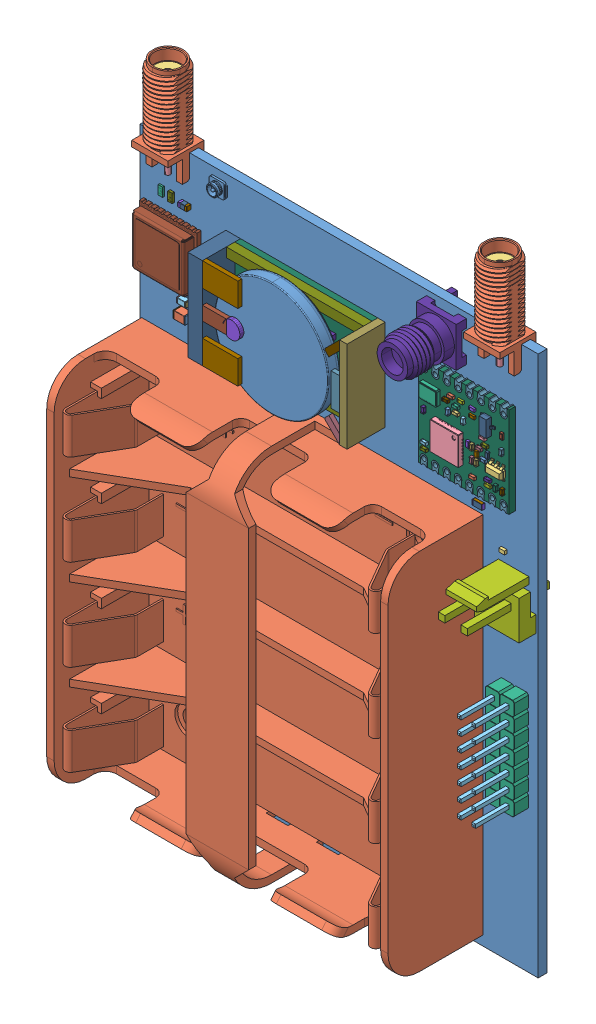
SolidWorks assembly Печатная плата Peggy Tracker, configuration Default. Lengths in mm. (continued)
Components (placement in the parent): (continued)
- Печатная плата Peggy Tracker(2)^Печатная плата Peggy Tracker-1: Печатная плата Peggy Tracker(2)^Печатная плата Peggy Tracker [Default] at origin size (70 108.1 20.64) (virtual) (continued)
  - DD2^Печатная плата Peggy Tracker(2)_Печатная плата Peggy Tracker-1: DD2^Печатная плата Peggy Tracker(2)_Печатная плата Peggy Tracker [Default] at origin size (15.9 16 2.23) (virtual) (continued)
    - User_Library-RFM96W^DD2_Печатная плата Peggy Tracker(2)_Печатная плата Peggy Tracker-1: User_Library-RFM96W^DD2_Печатная плата Peggy Tracker(2)_Печатная плата Peggy Tracker [Default] at (50.075 85.102 1.15) x (0 -1 0) z (0 0 1) size (16 15.9 2.23) (virtual) (continued)
      - Designator31^User_Library-RFM96W_DD2_Печатная плата Peggy Tracker(2)_Печатная плата Peggy Tracker-1: Designator31^User_Library-RFM96W_DD2_Печатная плата Peggy Tracker(2)_Печатная плата Peggy Tracker [Default] at origin size (1 0.5 0.5) (virtual) (continued)
        - Cap0402^Designator31_User_Library-RFM96W_DD2_Печатная плата Peggy Tracker(2)_Печатная плата Peggy Tracker-1: Cap0402^Designator31_User_Library-RFM96W_DD2_Печатная плата Peggy Tracker(2)_Печатная плата Peggy Tracker [По умолчанию] at (8.636 9.652 0) x (-1 0 0) z (0 1 0) size (1 0.5 0.5) (virtual)
      - Designator32^User_Library-RFM96W_DD2_Печатная плата Peggy Tracker(2)_Печатная плата Peggy Tracker-1: Designator32^User_Library-RFM96W_DD2_Печатная плата Peggy Tracker(2)_Печатная плата Peggy Tracker [Default] at origin size (1 0.5 0.5) (virtual)
        - Cap0402^Designator32_User_Library-RFM96W_DD2_Печатная плата Peggy Tracker(2)_Печатная плата Peggy Tracker-1: Cap0402^Designator32_User_Library-RFM96W_DD2_Печатная плата Peggy Tracker(2)_Печатная плата Peggy Tracker [По умолчанию] at (10.668 9.652 0) x (-1 0 0) z (0 1 0) size (1 0.5 0.5) (virtual)
      - Free-Models^User_Library-RFM96W_DD2_Печатная плата Peggy Tracker(2)_Печатная плата Peggy Tracker-1: Free-Models^User_Library-RFM96W_DD2_Печатная плата Peggy Tracker(2)_Печатная плата Peggy Tracker [Default] at origin size (16 15.3 1.16) (virtual)
        - Goldcontact^Free-Models_User_Library-RFM96W_DD2_Печатная плата Peggy Tracker(2)_Печатная плата Peggy Tracker-1: Goldcontact^Free-Models_User_Library-RFM96W_DD2_Печатная плата Peggy Tracker(2)_Печатная плата Peggy Tracker [По умолчанию] at (0.56 1 -1.14) x (-1 0 0) z (0 1 0) size (1.77 1.16 1.3) (virtual)
        - Goldcontact^Free-Models_User_Library-RFM96W_DD2_Печатная плата Peggy Tracker(2)_Печатная плата Peggy Tracker-2: Goldcontact^Free-Models_User_Library-RFM96W_DD2_Печатная плата Peggy Tracker(2)_Печатная плата Peggy Tracker [По умолчанию] at (0.56 3 -1.14) x (-1 0 0) z (0 1 0) size (1.77 1.16 1.3) (virtual)
        - Goldcontact^Free-Models_User_Library-RFM96W_DD2_Печатная плата Peggy Tracker(2)_Печатная плата Peggy Tracker-3: Goldcontact^Free-Models_User_Library-RFM96W_DD2_Печатная плата Peggy Tracker(2)_Печатная плата Peggy Tracker [По умолчанию] at (0.56 5 -1.14) x (-1 0 0) z (0 1 0) size (1.77 1.16 1.3) (virtual)
        - Goldcontact^Free-Models_User_Library-RFM96W_DD2_Печатная плата Peggy Tracker(2)_Печатная плата Peggy Tracker-4: Goldcontact^Free-Models_User_Library-RFM96W_DD2_Печатная плата Peggy Tracker(2)_Печатная плата Peggy Tracker [По умолчанию] at (0.56 7 -1.14) x (-1 0 0) z (0 1 0) size (1.77 1.16 1.3) (virtual)
        - Goldcontact^Free-Models_User_Library-RFM96W_DD2_Печатная плата Peggy Tracker(2)_Печатная плата Peggy Tracker-5: Goldcontact^Free-Models_User_Library-RFM96W_DD2_Печатная плата Peggy Tracker(2)_Печатная плата Peggy Tracker [По умолчанию] at (0.56 9 -1.14) x (-1 0 0) z (0 1 0) size (1.77 1.16 1.3) (virtual)
        - Goldcontact^Free-Models_User_Library-RFM96W_DD2_Печатная плата Peggy Tracker(2)_Печатная плата Peggy Tracker-6: Goldcontact^Free-Models_User_Library-RFM96W_DD2_Печатная плата Peggy Tracker(2)_Печатная плата Peggy Tracker [По умолчанию] at (0.56 11 -1.14) x (-1 0 0) z (0 1 0) size (1.77 1.16 1.3) (virtual)
        - Goldcontact^Free-Models_User_Library-RFM96W_DD2_Печатная плата Peggy Tracker(2)_Печатная плата Peggy Tracker-7: Goldcontact^Free-Models_User_Library-RFM96W_DD2_Печатная плата Peggy Tracker(2)_Печатная плата Peggy Tracker [По умолчанию] at (0.56 13 -1.14) x (-1 0 0) z (0 1 0) size (1.77 1.16 1.3) (virtual)
        - Goldcontact^Free-Models_User_Library-RFM96W_DD2_Печатная плата Peggy Tracker(2)_Печатная плата Peggy Tracker-8: Goldcontact^Free-Models_User_Library-RFM96W_DD2_Печатная плата Peggy Tracker(2)_Печатная плата Peggy Tracker [По умолчанию] at (0.56 15 -1.14) x (-1 0 0) z (0 1 0) size (1.77 1.16 1.3) (virtual)
        - Goldcontact^Free-Models_User_Library-RFM96W_DD2_Печатная плата Peggy Tracker(2)_Печатная плата Peggy Tracker-9: Goldcontact^Free-Models_User_Library-RFM96W_DD2_Печатная плата Peggy Tracker(2)_Печатная плата Peggy Tracker [По умолчанию] at (15.442 15 -1.14) x (1 0 0) z (0 -1 0) size (1.77 1.16 1.3) (virtual)
        - Goldcontact^Free-Models_User_Library-RFM96W_DD2_Печатная плата Peggy Tracker(2)_Печатная плата Peggy Tracker-10: Goldcontact^Free-Models_User_Library-RFM96W_DD2_Печатная плата Peggy Tracker(2)_Печатная плата Peggy Tracker [По умолчанию] at (15.442 13 -1.14) x (1 0 0) z (0 -1 0) size (1.77 1.16 1.3) (virtual)
        - Goldcontact^Free-Models_User_Library-RFM96W_DD2_Печатная плата Peggy Tracker(2)_Печатная плата Peggy Tracker-11: Goldcontact^Free-Models_User_Library-RFM96W_DD2_Печатная плата Peggy Tracker(2)_Печатная плата Peggy Tracker [По умолчанию] at (15.442 11 -1.14) x (1 0 0) z (0 -1 0) size (1.77 1.16 1.3) (virtual)
        - Goldcontact^Free-Models_User_Library-RFM96W_DD2_Печатная плата Peggy Tracker(2)_Печатная плата Peggy Tracker-12: Goldcontact^Free-Models_User_Library-RFM96W_DD2_Печатная плата Peggy Tracker(2)_Печатная плата Peggy Tracker [По умолчанию] at (15.442 9 -1.14) x (1 0 0) z (0 -1 0) size (1.77 1.16 1.3) (virtual)
        - Goldcontact^Free-Models_User_Library-RFM96W_DD2_Печатная плата Peggy Tracker(2)_Печатная плата Peggy Tracker-13: Goldcontact^Free-Models_User_Library-RFM96W_DD2_Печатная плата Peggy Tracker(2)_Печатная плата Peggy Tracker [По умолчанию] at (15.442 7 -1.14) x (1 0 0) z (0 -1 0) size (1.77 1.16 1.3) (virtual)
        - Goldcontact^Free-Models_User_Library-RFM96W_DD2_Печатная плата Peggy Tracker(2)_Печатная плата Peggy Tracker-14: Goldcontact^Free-Models_User_Library-RFM96W_DD2_Печатная плата Peggy Tracker(2)_Печатная плата Peggy Tracker [По умолчанию] at (15.442 5 -1.14) x (1 0 0) z (0 -1 0) size (1.77 1.16 1.3) (virtual)
        - Goldcontact^Free-Models_User_Library-RFM96W_DD2_Печатная плата Peggy Tracker(2)_Печатная плата Peggy Tracker-15: Goldcontact^Free-Models_User_Library-RFM96W_DD2_Печатная плата Peggy Tracker(2)_Печатная плата Peggy Tracker [По умолчанию] at (15.442 3 -1.14) x (1 0 0) z (0 -1 0) size (1.77 1.16 1.3) (virtual)
        - Goldcontact^Free-Models_User_Library-RFM96W_DD2_Печатная плата Peggy Tracker(2)_Печатная плата Peggy Tracker-16: Goldcontact^Free-Models_User_Library-RFM96W_DD2_Печатная плата Peggy Tracker(2)_Печатная плата Peggy Tracker [По умолчанию] at (15.442 1 -1.14) x (1 0 0) z (0 -1 0) size (1.77 1.16 1.3) (virtual)
      - Board-15^User_Library-RFM96W_DD2_Печатная плата Peggy Tracker(2)_Печатная плата Peggy Tracker-1: Board-15^User_Library-RFM96W_DD2_Печатная плата Peggy Tracker(2)_Печатная плата Peggy Tracker [По умолчанию] at (0 0 -1.1204) size (15.9 15.9 1.12) (virtual)
  - D2^Печатная плата Peggy Tracker(2)_Печатная плата Peggy Tracker-1: D2^Печатная плата Peggy Tracker(2)_Печатная плата Peggy Tracker [Default] at origin size (4.9 6 1.75) (virtual)
    - User_Library-SOIC-8-1^D2_Печатная плата Peggy Tracker(2)_Печатная плата Peggy Tracker-1: User_Library-SOIC-8-1^D2_Печатная плата Peggy Tracker(2)_Печатная плата Peggy Tracker [По умолчанию] at (19.8999 49.3999 -1.5596) x (1 0 0) z (0 0 -1) size (4.9 6 1.75) (virtual)
  - D1^Печатная плата Peggy Tracker(2)_Печатная плата Peggy Tracker-1: D1^Печатная плата Peggy Tracker(2)_Печатная плата Peggy Tracker [Default] at origin size (6.6 6.6 1.2) (virtual)
    - TSSOP-20^D1_Печатная плата Peggy Tracker(2)_Печатная плата Peggy Tracker-1: TSSOP-20^D1_Печатная плата Peggy Tracker(2)_Печатная плата Peggy Tracker [По умолчанию] at (14.6001 18.2999 -1.5596) x (0 1 0) z (-1 0 0) size (6.6 1.2 6.6) (virtual)
  - C15^Печатная плата Peggy Tracker(2)_Печатная плата Peggy Tracker-1: C15^Печатная плата Peggy Tracker(2)_Печатная плата Peggy Tracker [Default] at origin size (1.6 3.2 1) (virtual)
    - SW3dPS-1206_SMD_Capacitor^C15_Печатная плата Peggy Tracker(2)_Печатная плата Peggy Tracker-1: SW3dPS-1206_SMD_Capacitor^C15_Печатная плата Peggy Tracker(2)_Печатная плата Peggy Tracker [По умолчанию] at (29.1 17.2 -1.5596) x (0 -1 0) z (1 0 0) size (3.2 1 1.6) (virtual)
  - C14^Печатная плата Peggy Tracker(2)_Печатная плата Peggy Tracker-1: C14^Печатная плата Peggy Tracker(2)_Печатная плата Peggy Tracker [Default] at origin size (3.2 1.6 1) (virtual)
    - SW3dPS-1206_SMD_Capacitor^C14_Печатная плата Peggy Tracker(2)_Печатная плата Peggy Tracker-1: SW3dPS-1206_SMD_Capacitor^C14_Печатная плата Peggy Tracker(2)_Печатная плата Peggy Tracker [По умолчанию] at (58.6 84.5 -1.5596) x (1 0 0) z (0 1 0) size (3.2 1 1.6) (virtual)
  - C13^Печатная плата Peggy Tracker(2)_Печатная плата Peggy Tracker-1: C13^Печатная плата Peggy Tracker(2)_Печатная плата Peggy Tracker [Default] at origin size (0.8 1.6 0.3) (virtual)
    - SW3dPS-0603_SMD_Capacitor^C13_Печатная плата Peggy Tracker(2)_Печатная плата Peggy Tracker-1: SW3dPS-0603_SMD_Capacitor^C13_Печатная плата Peggy Tracker(2)_Печатная плата Peggy Tracker [По умолчанию] at (15.5001 55.6001 -1.5596) x (0 1 0) z (-1 0 0) size (1.6 0.3 0.8) (virtual)
  - C12^Печатная плата Peggy Tracker(2)_Печатная плата Peggy Tracker-1: C12^Печатная плата Peggy Tracker(2)_Печатная плата Peggy Tracker [Default] at origin size (0.8 1.6 0.3) (virtual)
    - SW3dPS-0603_SMD_Capacitor^C12_Печатная плата Peggy Tracker(2)_Печатная плата Peggy Tracker-1: SW3dPS-0603_SMD_Capacitor^C12_Печатная плата Peggy Tracker(2)_Печатная плата Peggy Tracker [По умолчанию] at (21.6999 54.9999 -1.5596) x (0 -1 0) z (1 0 0) size (1.6 0.3 0.8) (virtual)
  - C11^Печатная плата Peggy Tracker(2)_Печатная плата Peggy Tracker-1: C11^Печатная плата Peggy Tracker(2)_Печатная плата Peggy Tracker [Default] at origin size (1.7 0.9 0.9) (virtual)
    - 5945466272^C11_Печатная плата Peggy Tracker(2)_Печатная плата Peggy Tracker-1: 5945466272^C11_Печатная плата Peggy Tracker(2)_Печатная плата Peggy Tracker [Default] at (17.1 44.6 -1.5596) x (1 0 0) z (0 0 -1) size (1.7 0.9 0.9) (virtual)
      - Terminal-3^5945466272_C11_Печатная плата Peggy Tracker(2)_Печатная плата Peggy Tracker-1: Terminal-3^5945466272_C11_Печатная плата Peggy Tracker(2)_Печатная плата Peggy Tracker [Default] at (-0.85 -0.45 0) size (1.7 0.9 0.9) (virtual)
        - Open_CASCADE_STEP_translator_6.8_5.1.1^Terminal-3_5945466272_C11_Печатная плата Peggy Tracker(2)_Печатная плата Peggy Tracker-1: Open_CASCADE_STEP_translator_6.8_5.1.1^Terminal-3_5945466272_C11_Печатная плата Peggy Tracker(2)_Печатная плата Peggy Tracker [По умолчанию] at origin size (0.2 0.9 0.9) (virtual)
        - Open_CASCADE_STEP_translator_6.8_5.1.2^Terminal-3_5945466272_C11_Печатная плата Peggy Tracker(2)_Печатная плата Peggy Tracker-1: Open_CASCADE_STEP_translator_6.8_5.1.2^Terminal-3_5945466272_C11_Печатная плата Peggy Tracker(2)_Печатная плата Peggy Tracker [По умолчанию] at origin size (0.2 0.9 0.9) (virtual)
      - Mid_Body-1^5945466272_C11_Печатная плата Peggy Tracker(2)_Печатная плата Peggy Tracker-1: Mid_Body-1^5945466272_C11_Печатная плата Peggy Tracker(2)_Печатная плата Peggy Tracker [Default] at (-0.85 -0.45 0) size (1.3 0.9 0.9) (virtual)
        - Open_CASCADE_STEP_translator_6.8_5.2.1^Mid_Body-1_5945466272_C11_Печатная плата Peggy Tracker(2)_Печатная плата Peggy Tracker-1: Open_CASCADE_STEP_translator_6.8_5.2.1^Mid_Body-1_5945466272_C11_Печатная плата Peggy Tracker(2)_Печатная плата Peggy Tracker [По умолчанию] at origin size (1.3 0.9 0.9) (virtual)
  - C10^Печатная плата Peggy Tracker(2)_Печатная плата Peggy Tracker-1: C10^Печатная плата Peggy Tracker(2)_Печатная плата Peggy Tracker [Default] at origin size (1.75 0.95 0.87) (virtual)
    - 5945472432^C10_Печатная плата Peggy Tracker(2)_Печатная плата Peggy Tracker-1: 5945472432^C10_Печатная плата Peggy Tracker(2)_Печатная плата Peggy Tracker [Default] at (20.5 34.6 -1.5596) x (-1 0 0) z (0 0 -1) size (1.75 0.95 0.87) (virtual)
      - Terminal-4^5945472432_C10_Печатная плата Peggy Tracker(2)_Печатная плата Peggy Tracker-1: Terminal-4^5945472432_C10_Печатная плата Peggy Tracker(2)_Печатная плата Peggy Tracker [Default] at (-0.875 -0.475 0) size (1.75 0.95 0.87) (virtual)
        - Open_CASCADE_STEP_translator_6.8_127.1.1^Terminal-4_5945472432_C10_Печатная плата Peggy Tracker(2)_Печатная плата Peggy Tracker-1: Open_CASCADE_STEP_translator_6.8_127.1.1^Terminal-4_5945472432_C10_Печатная плата Peggy Tracker(2)_Печатная плата Peggy Tracker [По умолчанию] at origin size (0.2 0.95 0.87) (virtual)
        - Open_CASCADE_STEP_translator_6.8_127.1.2^Terminal-4_5945472432_C10_Печатная плата Peggy Tracker(2)_Печатная плата Peggy Tracker-1: Open_CASCADE_STEP_translator_6.8_127.1.2^Terminal-4_5945472432_C10_Печатная плата Peggy Tracker(2)_Печатная плата Peggy Tracker [По умолчанию] at origin size (0.2 0.95 0.87) (virtual)
      - Mid_Body-2^5945472432_C10_Печатная плата Peggy Tracker(2)_Печатная плата Peggy Tracker-1: Mid_Body-2^5945472432_C10_Печатная плата Peggy Tracker(2)_Печатная плата Peggy Tracker [Default] at (-0.875 -0.475 0) size (1.35 0.95 0.87) (virtual)
        - Open_CASCADE_STEP_translator_6.8_127.2.1^Mid_Body-2_5945472432_C10_Печатная плата Peggy Tracker(2)_Печатная плата Peggy Tracker-1: Open_CASCADE_STEP_translator_6.8_127.2.1^Mid_Body-2_5945472432_C10_Печатная плата Peggy Tracker(2)_Печатная плата Peggy Tracker [По умолчанию] at origin size (1.35 0.95 0.87) (virtual)
  - C9^Печатная плата Peggy Tracker(2)_Печатная плата Peggy Tracker-1: C9^Печатная плата Peggy Tracker(2)_Печатная плата Peggy Tracker [Default] at origin size (1.75 0.95 0.87) (virtual)
    - 5945463072^C9_Печатная плата Peggy Tracker(2)_Печатная плата Peggy Tracker-1: 5945463072^C9_Печатная плата Peggy Tracker(2)_Печатная плата Peggy Tracker [Default] at (22 42.9 -1.5596) x (1 0 0) z (0 0 -1) size (1.75 0.95 0.87) (virtual)
      - Terminal-5^5945463072_C9_Печатная плата Peggy Tracker(2)_Печатная плата Peggy Tracker-1: Terminal-5^5945463072_C9_Печатная плата Peggy Tracker(2)_Печатная плата Peggy Tracker [Default] at (-0.875 -0.475 0) size (1.75 0.95 0.87) (virtual)
        - Open_CASCADE_STEP_translator_6.8_127.1.1-16^Terminal-5_5945463072_C9_Печатная плата Peggy Tracker(2)_Печатная плата Peggy Tracker-1: Open_CASCADE_STEP_translator_6.8_127.1.1-16^Terminal-5_5945463072_C9_Печатная плата Peggy Tracker(2)_Печатная плата Peggy Tracker [По умолчанию] at origin size (0.2 0.95 0.87) (virtual)
        - Open_CASCADE_STEP_translator_6.8_127.1.2-17^Terminal-5_5945463072_C9_Печатная плата Peggy Tracker(2)_Печатная плата Peggy Tracker-1: Open_CASCADE_STEP_translator_6.8_127.1.2-17^Terminal-5_5945463072_C9_Печатная плата Peggy Tracker(2)_Печатная плата Peggy Tracker [По умолчанию] at origin size (0.2 0.95 0.87) (virtual)
      - Mid_Body-3^5945463072_C9_Печатная плата Peggy Tracker(2)_Печатная плата Peggy Tracker-1: Mid_Body-3^5945463072_C9_Печатная плата Peggy Tracker(2)_Печатная плата Peggy Tracker [Default] at (-0.875 -0.475 0) size (1.35 0.95 0.87) (virtual)
        - Open_CASCADE_STEP_translator_6.8_127.2.1-18^Mid_Body-3_5945463072_C9_Печатная плата Peggy Tracker(2)_Печатная плата Peggy Tracker-1: Open_CASCADE_STEP_translator_6.8_127.2.1-18^Mid_Body-3_5945463072_C9_Печатная плата Peggy Tracker(2)_Печатная плата Peggy Tracker [По умолчанию] at origin size (1.35 0.95 0.87) (virtual)
  - C8^Печатная плата Peggy Tracker(2)_Печатная плата Peggy Tracker-1: C8^Печатная плата Peggy Tracker(2)_Печатная плата Peggy Tracker [Default] at origin size (1.25 2 0.78) (virtual)
    - SW3dPS-0805_SMD_Capacitor^C8_Печатная плата Peggy Tracker(2)_Печатная плата Peggy Tracker-1: SW3dPS-0805_SMD_Capacitor^C8_Печатная плата Peggy Tracker(2)_Печатная плата Peggy Tracker [По умолчанию] at (20.3001 21.6001 -1.5596) x (0 1 0) z (-1 0 0) size (2 0.78 1.25) (virtual)
  - C7^Печатная плата Peggy Tracker(2)_Печатная плата Peggy Tracker-1: C7^Печатная плата Peggy Tracker(2)_Печатная плата Peggy Tracker [Default] at origin size (1.6 3.2 1) (virtual)
    - SW3dPS-1206_SMD_Capacitor^C7_Печатная плата Peggy Tracker(2)_Печатная плата Peggy Tracker-1: SW3dPS-1206_SMD_Capacitor^C7_Печатная плата Peggy Tracker(2)_Печатная плата Peggy Tracker [По умолчанию] at (6.9 17.8 -1.5596) x (0 -1 0) z (1 0 0) size (3.2 1 1.6) (virtual)
  - C6^Печатная плата Peggy Tracker(2)_Печатная плата Peggy Tracker-1: C6^Печатная плата Peggy Tracker(2)_Печатная плата Peggy Tracker [Default] at origin size (1.25 2 0.78) (virtual)
    - SW3dPS-0805_SMD_Capacitor^C6_Печатная плата Peggy Tracker(2)_Печатная плата Peggy Tracker-1: SW3dPS-0805_SMD_Capacitor^C6_Печатная плата Peggy Tracker(2)_Печатная плата Peggy Tracker [По умолчанию] at (9.3262 19.274 -1.5596) x (0 1 0) z (-1 0 0) size (2 0.78 1.25) (virtual)
  - C5^Печатная плата Peggy Tracker(2)_Печатная плата Peggy Tracker-1: C5^Печатная плата Peggy Tracker(2)_Печатная плата Peggy Tracker [Default] at origin size (1.6 3.2 1) (virtual)
    - SW3dPS-1206_SMD_Capacitor^C5_Печатная плата Peggy Tracker(2)_Печатная плата Peggy Tracker-1: SW3dPS-1206_SMD_Capacitor^C5_Печатная плата Peggy Tracker(2)_Печатная плата Peggy Tracker [По умолчанию] at (23.9 17.2 -1.5596) x (0 -1 0) z (1 0 0) size (3.2 1 1.6) (virtual)
  - C4^Печатная плата Peggy Tracker(2)_Печатная плата Peggy Tracker-1: C4^Печатная плата Peggy Tracker(2)_Печатная плата Peggy Tracker [Default] at origin size (1.6 3.2 1) (virtual)
    - SW3dPS-1206_SMD_Capacitor^C4_Печатная плата Peggy Tracker(2)_Печатная плата Peggy Tracker-1: SW3dPS-1206_SMD_Capacitor^C4_Печатная плата Peggy Tracker(2)_Печатная плата Peggy Tracker [По умолчанию] at (26.5 17.2 -1.5596) x (0 -1 0) z (1 0 0) size (3.2 1 1.6) (virtual)
  - C3^Печатная плата Peggy Tracker(2)_Печатная плата Peggy Tracker-1: C3^Печатная плата Peggy Tracker(2)_Печатная плата Peggy Tracker [Default] at origin size (2.1 1.35 1.35) (virtual)
    - 5945472512^C3_Печатная плата Peggy Tracker(2)_Печатная плата Peggy Tracker-1: 5945472512^C3_Печатная плата Peggy Tracker(2)_Печатная плата Peggy Tracker [Default] at (8.2 70.3 0) x (1 0 0) z (0 0 1) size (2.1 1.35 1.35) (virtual)
      - Terminal-6^5945472512_C3_Печатная плата Peggy Tracker(2)_Печатная плата Peggy Tracker-1: Terminal-6^5945472512_C3_Печатная плата Peggy Tracker(2)_Печатная плата Peggy Tracker [Default] at (-1.05 -0.675 0) size (2.1 1.35 1.35) (virtual)
        - Open_CASCADE_STEP_translator_6.8_24.1.1^Terminal-6_5945472512_C3_Печатная плата Peggy Tracker(2)_Печатная плата Peggy Tracker-1: Open_CASCADE_STEP_translator_6.8_24.1.1^Terminal-6_5945472512_C3_Печатная плата Peggy Tracker(2)_Печатная плата Peggy Tracker [По умолчанию] at origin size (0.2 1.35 1.35) (virtual)
        - Open_CASCADE_STEP_translator_6.8_24.1.2^Terminal-6_5945472512_C3_Печатная плата Peggy Tracker(2)_Печатная плата Peggy Tracker-1: Open_CASCADE_STEP_translator_6.8_24.1.2^Terminal-6_5945472512_C3_Печатная плата Peggy Tracker(2)_Печатная плата Peggy Tracker [По умолчанию] at origin size (0.2 1.35 1.35) (virtual)
      - Mid_Body-4^5945472512_C3_Печатная плата Peggy Tracker(2)_Печатная плата Peggy Tracker-1: Mid_Body-4^5945472512_C3_Печатная плата Peggy Tracker(2)_Печатная плата Peggy Tracker [Default] at (-1.05 -0.675 0) size (1.7 1.35 1.35) (virtual)
        - Open_CASCADE_STEP_translator_6.8_24.2.1^Mid_Body-4_5945472512_C3_Печатная плата Peggy Tracker(2)_Печатная плата Peggy Tracker-1: Open_CASCADE_STEP_translator_6.8_24.2.1^Mid_Body-4_5945472512_C3_Печатная плата Peggy Tracker(2)_Печатная плата Peggy Tracker [По умолчанию] at origin size (1.7 1.35 1.35) (virtual)
  - C2^Печатная плата Peggy Tracker(2)_Печатная плата Peggy Tracker-1: C2^Печатная плата Peggy Tracker(2)_Печатная плата Peggy Tracker [Default] at origin size (1.7 0.9 0.9) (virtual)
    - 5945463872^C2_Печатная плата Peggy Tracker(2)_Печатная плата Peggy Tracker-1: 5945463872^C2_Печатная плата Peggy Tracker(2)_Печатная плата Peggy Tracker [Default] at (8.1 72.3 0) x (-1 0 0) z (0 0 1) size (1.7 0.9 0.9) (virtual)
      - Terminal-7^5945463872_C2_Печатная плата Peggy Tracker(2)_Печатная плата Peggy Tracker-1: Terminal-7^5945463872_C2_Печатная плата Peggy Tracker(2)_Печатная плата Peggy Tracker [Default] at (-0.85 -0.45 0) size (1.7 0.9 0.9) (virtual)
        - Open_CASCADE_STEP_translator_6.8_5.1.1-19^Terminal-7_5945463872_C2_Печатная плата Peggy Tracker(2)_Печатная плата Peggy Tracker-1: Open_CASCADE_STEP_translator_6.8_5.1.1-19^Terminal-7_5945463872_C2_Печатная плата Peggy Tracker(2)_Печатная плата Peggy Tracker [По умолчанию] at origin size (0.2 0.9 0.9) (virtual)
        - Open_CASCADE_STEP_translator_6.8_5.1.2-20^Terminal-7_5945463872_C2_Печатная плата Peggy Tracker(2)_Печатная плата Peggy Tracker-1: Open_CASCADE_STEP_translator_6.8_5.1.2-20^Terminal-7_5945463872_C2_Печатная плата Peggy Tracker(2)_Печатная плата Peggy Tracker [По умолчанию] at origin size (0.2 0.9 0.9) (virtual)
      - Mid_Body-5^5945463872_C2_Печатная плата Peggy Tracker(2)_Печатная плата Peggy Tracker-1: Mid_Body-5^5945463872_C2_Печатная плата Peggy Tracker(2)_Печатная плата Peggy Tracker [Default] at (-0.85 -0.45 0) size (1.3 0.9 0.9) (virtual)
        - Open_CASCADE_STEP_translator_6.8_5.2.1-21^Mid_Body-5_5945463872_C2_Печатная плата Peggy Tracker(2)_Печатная плата Peggy Tracker-1: Open_CASCADE_STEP_translator_6.8_5.2.1-21^Mid_Body-5_5945463872_C2_Печатная плата Peggy Tracker(2)_Печатная плата Peggy Tracker [По умолчанию] at origin size (1.3 0.9 0.9) (virtual)
  - C1^Печатная плата Peggy Tracker(2)_Печатная плата Peggy Tracker-1: C1^Печатная плата Peggy Tracker(2)_Печатная плата Peggy Tracker [Default] at origin size (0.8 1.6 0.3) (virtual)
    - SW3dPS-0603_SMD_Capacitor^C1_Печатная плата Peggy Tracker(2)_Печатная плата Peggy Tracker-1: SW3dPS-0603_SMD_Capacitor^C1_Печатная плата Peggy Tracker(2)_Печатная плата Peggy Tracker [По умолчанию] at (3.8752 86.9 0) x (0 -1 0) z (-1 0 0) size (1.6 0.3 0.8) (virtual)
